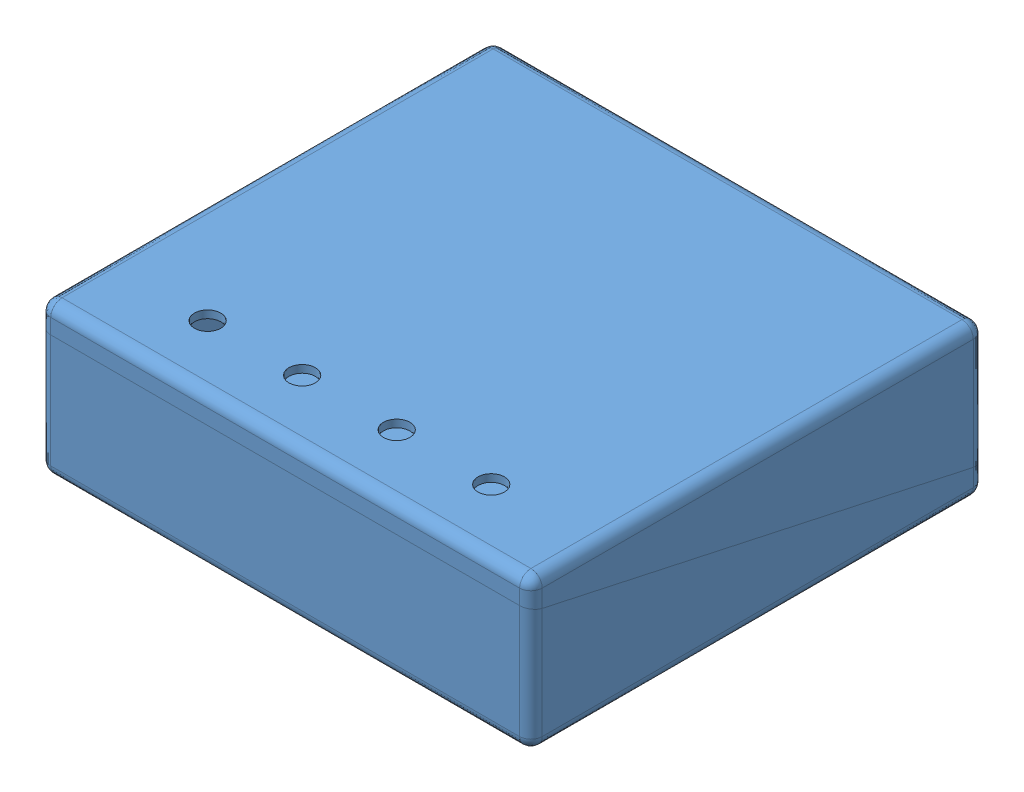
SolidWorks assembly carcasa_assembly, configuration Default. Lengths in mm.
Overall size (130 40.54 120).
283 component instances, 32 part files, 6 mates.
Components (placement in the parent):
- caracasa_amp-1: caracasa_amp [Default] at (26.1014 72.6802 108.3315) size (130 40 120)
- basic_digital1-basic_digital.step-1: basic_digital1-basic_digital.step [Default] at (-122.8986 98.8802 119.3315) x (1 0 0) z (0 1 0) size (102.24 56.26 11.54)
  - Board_Geoms_72f.step-1: Board_Geoms_72f.step [Default] at origin size (90 55 1.59)
    - Pcb_72f.step-1: Pcb_72f.step [Default] at origin size (90 55 1.59)
  - Step_Models_72f.step-1: Step_Models_72f.step [Default] at origin size (102.24 49.36 11.54)
    - Top_72f.step-1: Top_72f.step [Default] at origin size (102.24 49.36 11.54)
      - IC3_ASSEMBLY_e554ddd5023d.step-1: IC3_ASSEMBLY_e554ddd5023d.step [Default] at (179.75 26.5 0) x (0 1 0) z (0 0 1) size (5 4.4 1.3)
        - Body.step-1: Body.step [Default] at (0 0 0.1) size (5 4.4 1.2)
        - Pins.step-1: Pins.step [Default] at origin size (4.21 4.36 0.1)
      - IC1_DPD0012A_ASM_3e18ce07ad7c.step-1: IC1_DPD0012A_ASM_3e18ce07ad7c.step [Default] at (149 25.01 0.05) x (1 0 0) z (0 -1 0) size (3 0.8 3)
        - BODY-SON.step-1: BODY-SON.step [Default] at origin size (3 0.75 3)
        - FRAME-DPD0012A.step-1: FRAME-DPD0012A.step [Default] at (0 -0.05 0) size (3 0.2 3)
      - IC2_D0008A_ASM_81426aa18051.step-1: IC2_D0008A_ASM_81426aa18051.step [Default] at (131 58 0) x (0 1 0) z (0 0 1) size (6.02 4.91 1.63)
        - BODY-SO.step-1: BODY-SO.step [Default] at (0 0 1.0033) x (0 1 0) z (1 0 0) size (4.91 1.45 3.92)
        - LEAD-D0008A.step-1: LEAD-D0008A.step [Default] at (2.159 1.905 0.254) x (0 1 0) z (1 0 0) size (0.42 1 1.06)
        - LEAD-D0008A.step-2: LEAD-D0008A.step [Default] at (2.159 0.635 0.254) x (0 1 0) z (1 0 0) size (0.42 1 1.06)
        - LEAD-D0008A.step-3: LEAD-D0008A.step [Default] at (2.159 -0.635 0.254) x (0 1 0) z (1 0 0) size (0.42 1 1.06)
        - LEAD-D0008A.step-4: LEAD-D0008A.step [Default] at (2.159 -1.905 0.254) x (0 1 0) z (1 0 0) size (0.42 1 1.06)
        - LEAD-D0008A.step-5: LEAD-D0008A.step [Default] at (-2.159 1.905 0.254) x (0 -1 0) z (-1 0 0) size (0.42 1 1.06)
        - LEAD-D0008A.step-6: LEAD-D0008A.step [Default] at (-2.159 0.635 0.254) x (0 -1 0) z (-1 0 0) size (0.42 1 1.06)
        - LEAD-D0008A.step-7: LEAD-D0008A.step [Default] at (-2.159 -0.635 0.254) x (0 -1 0) z (-1 0 0) size (0.42 1 1.06)
        - LEAD-D0008A.step-8: LEAD-D0008A.step [Default] at (-2.159 -1.905 0.254) x (0 -1 0) z (-1 0 0) size (0.42 1 1.06)
      - R23_R_0603_1608Metric_a283bdbe5e44.step-1: R23_R_0603_1608Metric_a283bdbe5e44.step [Default] at (131 31.48 0) x (-1 0 0) z (0 0 1) size (1.6 0.8 0.45)
      - C52_C_0603_1608Metric_5a1a808c49e1.step-1: C52_C_0603_1608Metric_5a1a808c49e1.step [Default] at (186.25 28.5 0) x (-1 0 0) z (0 0 1) size (1.6 0.8 0.8)
      - U4_TSSOP_20_44x65mm_P065mm_811bc58fadb8.step-1: U4_TSSOP_20_44x65mm_P065mm_811bc58fadb8.step [Default] at (121.3625 24.725 0) size (6.4 6.5 1.2)
      - C52_C_0603_1608Metric_5a1a808c49e1.step-2: C52_C_0603_1608Metric_5a1a808c49e1.step [Default] at (136.75 61.25 0) x (0 1 0) z (0 0 1) size (1.6 0.8 0.8)
      - C52_C_0603_1608Metric_5a1a808c49e1.step-3: C52_C_0603_1608Metric_5a1a808c49e1.step [Default] at (151.45 44.75 0) size (1.6 0.8 0.8)
      - U7_ESP32-WROOM-32_9a0432253470.step-1: U7_ESP32-WROOM-32_9a0432253470.step [Default] at (113.495 39.92 0) x (0 1 0) z (0 0 1) size (18 25.5 3.1)
      - C52_C_0603_1608Metric_5a1a808c49e1.step-4: C52_C_0603_1608Metric_5a1a808c49e1.step [Default] at (134.25 38 0) x (0 1 0) z (0 0 1) size (1.6 0.8 0.8)
      - R23_R_0603_1608Metric_a283bdbe5e44.step-2: R23_R_0603_1608Metric_a283bdbe5e44.step [Default] at (169 35 0) size (1.6 0.8 0.45)
      - FB1_C_0805_2012Metric_4ba0fd9e626e.step-1: FB1_C_0805_2012Metric_4ba0fd9e626e.step [Default] at (150.3 56.55 0) x (-1 0 0) z (0 0 1) size (2 1.25 1.25)
      - C52_C_0603_1608Metric_5a1a808c49e1.step-5: C52_C_0603_1608Metric_5a1a808c49e1.step [Default] at (139 25.2 0) x (0 -1 0) z (0 0 1) size (1.6 0.8 0.8)
      - R23_R_0603_1608Metric_a283bdbe5e44.step-3: R23_R_0603_1608Metric_a283bdbe5e44.step [Default] at (169 36.5 0) x (-1 0 0) z (0 0 1) size (1.6 0.8 0.45)
      - R23_R_0603_1608Metric_a283bdbe5e44.step-4: R23_R_0603_1608Metric_a283bdbe5e44.step [Default] at (120.5 29 0) x (-1 0 0) z (0 0 1) size (1.6 0.8 0.45)
      - Q2_SOT_23_d2a7eeff1b69.step-1: Q2_SOT_23_d2a7eeff1b69.step [Default] at (144.75 22 0) size (2.5 3 1.2)
      - C52_C_0603_1608Metric_5a1a808c49e1.step-6: C52_C_0603_1608Metric_5a1a808c49e1.step [Default] at (159 25.25 0) x (0 1 0) z (0 0 1) size (1.6 0.8 0.8)
      - R23_R_0603_1608Metric_a283bdbe5e44.step-5: R23_R_0603_1608Metric_a283bdbe5e44.step [Default] at (132.25 46.5 0) x (-1 0 0) z (0 0 1) size (1.6 0.8 0.45)
      - FB1_C_0805_2012Metric_4ba0fd9e626e.step-2: FB1_C_0805_2012Metric_4ba0fd9e626e.step [Default] at (125.5 39 0) x (0 1 0) z (0 0 1) size (2 1.25 1.25)
      - C52_C_0603_1608Metric_5a1a808c49e1.step-7: C52_C_0603_1608Metric_5a1a808c49e1.step [Default] at (126.8625 24.975 0) x (-1 0 0) z (0 0 1) size (1.6 0.8 0.8)
      - Y1_Crystal_SMD_3225-4Pin_3.2x2.5mm_101ec78cddaa.step-1: Y1_Crystal_SMD_3225-4Pin_3.2x2.5mm_101ec78cddaa.step [Default] at (153.9 59.65 0) size (3.2 2.5 0.64)
      - J5_PinHeader_2x03_P254mm_Vertical_340915476f9a.step-1: J5_PinHeader_2x03_P254mm_Vertical_340915476f9a.step [Default] at (190.29 54.54 0) x (0 -1 0) z (0 0 1) size (5.08 7.62 11.54)
      - C52_C_0603_1608Metric_5a1a808c49e1.step-8: C52_C_0603_1608Metric_5a1a808c49e1.step [Default] at (127.98 32.98 0) x (-1 0 0) z (0 0 1) size (1.6 0.8 0.8)
      - C52_C_0603_1608Metric_5a1a808c49e1.step-9: C52_C_0603_1608Metric_5a1a808c49e1.step [Default] at (149.75 28.45 0) x (0 1 0) z (0 0 1) size (1.6 0.8 0.8)
      - C52_C_0603_1608Metric_5a1a808c49e1.step-10: C52_C_0603_1608Metric_5a1a808c49e1.step [Default] at (126.8625 26.475 0) x (-1 0 0) z (0 0 1) size (1.6 0.8 0.8)
      - C52_C_0603_1608Metric_5a1a808c49e1.step-11: C52_C_0603_1608Metric_5a1a808c49e1.step [Default] at (138.25 58.25 0) x (0 -1 0) z (0 0 1) size (1.6 0.8 0.8)
      - C52_C_0603_1608Metric_5a1a808c49e1.step-12: C52_C_0603_1608Metric_5a1a808c49e1.step [Default] at (162.3 49.05 0) x (-1 0 0) z (0 0 1) size (1.6 0.8 0.8)
      - R23_R_0603_1608Metric_a283bdbe5e44.step-6: R23_R_0603_1608Metric_a283bdbe5e44.step [Default] at (193 54.75 0) x (0 -1 0) z (0 0 1) size (1.6 0.8 0.45)
      - R23_R_0603_1608Metric_a283bdbe5e44.step-7: R23_R_0603_1608Metric_a283bdbe5e44.step [Default] at (167.5 47.25 0) x (-1 0 0) z (0 0 1) size (1.6 0.8 0.45)
      - D1_D_SOD_123_ffc0e81b88b9.step-1: D1_D_SOD_123_ffc0e81b88b9.step [Default] at (127 64.25 0) x (0 1 0) z (0 0 1) size (3.8 1.6 1.25)
      - R23_R_0603_1608Metric_a283bdbe5e44.step-8: R23_R_0603_1608Metric_a283bdbe5e44.step [Default] at (170.5 47.25 0) size (1.6 0.8 0.45)
      - C52_C_0603_1608Metric_5a1a808c49e1.step-13: C52_C_0603_1608Metric_5a1a808c49e1.step [Default] at (139 21.95 0) x (0 -1 0) z (0 0 1) size (1.6 0.8 0.8)
      - R23_R_0603_1608Metric_a283bdbe5e44.step-9: R23_R_0603_1608Metric_a283bdbe5e44.step [Default] at (169.75 32.75 0) x (0 1 0) z (0 0 1) size (1.6 0.8 0.45)
      - Q2_SOT_23_d2a7eeff1b69.step-2: Q2_SOT_23_d2a7eeff1b69.step [Default] at (153.25 22 0) x (-1 0 0) z (0 0 1) size (2.5 3 1.2)
      - R23_R_0603_1608Metric_a283bdbe5e44.step-10: R23_R_0603_1608Metric_a283bdbe5e44.step [Default] at (190 28.5 0) x (0 1 0) z (0 0 1) size (1.6 0.8 0.45)
      - C52_C_0603_1608Metric_5a1a808c49e1.step-14: C52_C_0603_1608Metric_5a1a808c49e1.step [Default] at (155.45 42.4 0) x (0 -1 0) z (0 0 1) size (1.6 0.8 0.8)
      - C52_C_0603_1608Metric_5a1a808c49e1.step-15: C52_C_0603_1608Metric_5a1a808c49e1.step [Default] at (114.3375 28.475 0) size (1.6 0.8 0.8)
      - R23_R_0603_1608Metric_a283bdbe5e44.step-11: R23_R_0603_1608Metric_a283bdbe5e44.step [Default] at (131.5 44.25 0) x (0 1 0) z (0 0 1) size (1.6 0.8 0.45)
      - R23_R_0603_1608Metric_a283bdbe5e44.step-12: R23_R_0603_1608Metric_a283bdbe5e44.step [Default] at (182.5 51.5 0) x (0 -1 0) z (0 0 1) size (1.6 0.8 0.45)
      - C52_C_0603_1608Metric_5a1a808c49e1.step-16: C52_C_0603_1608Metric_5a1a808c49e1.step [Default] at (171.25 32.75 0) x (0 -1 0) z (0 0 1) size (1.6 0.8 0.8)
      - C52_C_0603_1608Metric_5a1a808c49e1.step-17: C52_C_0603_1608Metric_5a1a808c49e1.step [Default] at (141.5 55.75 0) x (0 1 0) z (0 0 1) size (1.6 0.8 0.8)
      - R23_R_0603_1608Metric_a283bdbe5e44.step-13: R23_R_0603_1608Metric_a283bdbe5e44.step [Default] at (170 58.5 0) size (1.6 0.8 0.45)
      - C52_C_0603_1608Metric_5a1a808c49e1.step-18: C52_C_0603_1608Metric_5a1a808c49e1.step [Default] at (168.25 32.75 0) x (0 1 0) z (0 0 1) size (1.6 0.8 0.8)
      - R23_R_0603_1608Metric_a283bdbe5e44.step-14: R23_R_0603_1608Metric_a283bdbe5e44.step [Default] at (160.75 64.75 0) size (1.6 0.8 0.45)
      - C52_C_0603_1608Metric_5a1a808c49e1.step-19: C52_C_0603_1608Metric_5a1a808c49e1.step [Default] at (154.35 56.05 0) x (0 -1 0) z (0 0 1) size (1.6 0.8 0.8)
      - R23_R_0603_1608Metric_a283bdbe5e44.step-15: R23_R_0603_1608Metric_a283bdbe5e44.step [Default] at (170.5 48.75 0) x (-1 0 0) z (0 0 1) size (1.6 0.8 0.45)
      - R23_R_0603_1608Metric_a283bdbe5e44.step-16: R23_R_0603_1608Metric_a283bdbe5e44.step [Default] at (167.5 45.75 0) size (1.6 0.8 0.45)
      - C52_C_0603_1608Metric_5a1a808c49e1.step-20: C52_C_0603_1608Metric_5a1a808c49e1.step [Default] at (119 55.75 0) x (0 -1 0) z (0 0 1) size (1.6 0.8 0.8)
      - R23_R_0603_1608Metric_a283bdbe5e44.step-17: R23_R_0603_1608Metric_a283bdbe5e44.step [Default] at (130.25 33.75 0) x (0 -1 0) z (0 0 1) size (1.6 0.8 0.45)
      - C52_C_0603_1608Metric_5a1a808c49e1.step-21: C52_C_0603_1608Metric_5a1a808c49e1.step [Default] at (153.95 42.4 0) x (0 -1 0) z (0 0 1) size (1.6 0.8 0.8)
      - C52_C_0603_1608Metric_5a1a808c49e1.step-22: C52_C_0603_1608Metric_5a1a808c49e1.step [Default] at (142 25.2 0) x (0 1 0) z (0 0 1) size (1.6 0.8 0.8)
      - C52_C_0603_1608Metric_5a1a808c49e1.step-23: C52_C_0603_1608Metric_5a1a808c49e1.step [Default] at (126.8625 27.975 0) x (-1 0 0) z (0 0 1) size (1.6 0.8 0.8)
      - R23_R_0603_1608Metric_a283bdbe5e44.step-18: R23_R_0603_1608Metric_a283bdbe5e44.step [Default] at (170 64.5 0) size (1.6 0.8 0.45)
      - C52_C_0603_1608Metric_5a1a808c49e1.step-24: C52_C_0603_1608Metric_5a1a808c49e1.step [Default] at (150.51 21.5 0) x (0 1 0) z (0 0 1) size (1.6 0.8 0.8)
      - J2_PinHeader_1x05_P254mm_Vertical_afd68b060886.step-1: J2_PinHeader_1x05_P254mm_Vertical_afd68b060886.step [Default] at (154.04 64.5 0) x (0 -1 0) z (0 0 1) size (2.54 12.7 11.54)
      - C52_C_0603_1608Metric_5a1a808c49e1.step-25: C52_C_0603_1608Metric_5a1a808c49e1.step [Default] at (161.45 42.4 0) x (0 1 0) z (0 0 1) size (1.6 0.8 0.8)
      - C52_C_0603_1608Metric_5a1a808c49e1.step-26: C52_C_0603_1608Metric_5a1a808c49e1.step [Default] at (105.75 28.75 0) x (-1 0 0) z (0 0 1) size (1.6 0.8 0.8)
      - U1_LQFP_48_7x7mm_P05mm_03b825850876.step-1: U1_LQFP_48_7x7mm_P05mm_03b825850876.step [Default] at (163 58.5 0) size (9 9 1.5)
      - R23_R_0603_1608Metric_a283bdbe5e44.step-19: R23_R_0603_1608Metric_a283bdbe5e44.step [Default] at (134.6 64.825 0) x (0 1 0) z (0 0 1) size (1.6 0.8 0.45)
      - C52_C_0603_1608Metric_5a1a808c49e1.step-27: C52_C_0603_1608Metric_5a1a808c49e1.step [Default] at (172.75 49.5 0) x (0 -1 0) z (0 0 1) size (1.6 0.8 0.8)
      - C52_C_0603_1608Metric_5a1a808c49e1.step-28: C52_C_0603_1608Metric_5a1a808c49e1.step [Default] at (168 53.75 0) size (1.6 0.8 0.8)
      - R23_R_0603_1608Metric_a283bdbe5e44.step-20: R23_R_0603_1608Metric_a283bdbe5e44.step [Default] at (125.25 20.2 0) size (1.6 0.8 0.45)
      - C52_C_0603_1608Metric_5a1a808c49e1.step-29: C52_C_0603_1608Metric_5a1a808c49e1.step [Default] at (193 51.5 0) x (0 -1 0) z (0 0 1) size (1.6 0.8 0.8)
      - R23_R_0603_1608Metric_a283bdbe5e44.step-21: R23_R_0603_1608Metric_a283bdbe5e44.step [Default] at (170.5 50.25 0) x (-1 0 0) z (0 0 1) size (1.6 0.8 0.45)
      - C52_C_0603_1608Metric_5a1a808c49e1.step-30: C52_C_0603_1608Metric_5a1a808c49e1.step [Default] at (168.25 49.5 0) x (0 1 0) z (0 0 1) size (1.6 0.8 0.8)
      - C52_C_0603_1608Metric_5a1a808c49e1.step-31: C52_C_0603_1608Metric_5a1a808c49e1.step [Default] at (116.5875 27.725 0) x (0 1 0) z (0 0 1) size (1.6 0.8 0.8)
      - R23_R_0603_1608Metric_a283bdbe5e44.step-22: R23_R_0603_1608Metric_a283bdbe5e44.step [Default] at (159.95 42.4 0) x (0 -1 0) z (0 0 1) size (1.6 0.8 0.45)
      - R23_R_0603_1608Metric_a283bdbe5e44.step-23: R23_R_0603_1608Metric_a283bdbe5e44.step [Default] at (105 52.25 0) x (0 -1 0) z (0 0 1) size (1.6 0.8 0.45)
      - C52_C_0603_1608Metric_5a1a808c49e1.step-32: C52_C_0603_1608Metric_5a1a808c49e1.step [Default] at (151.45 49.4 0) x (-1 0 0) z (0 0 1) size (1.6 0.8 0.8)
      - R23_R_0603_1608Metric_a283bdbe5e44.step-24: R23_R_0603_1608Metric_a283bdbe5e44.step [Default] at (157.5 22.25 0) x (0 -1 0) z (0 0 1) size (1.6 0.8 0.45)
      - R23_R_0603_1608Metric_a283bdbe5e44.step-25: R23_R_0603_1608Metric_a283bdbe5e44.step [Default] at (108.25 28 0) x (0 -1 0) z (0 0 1) size (1.6 0.8 0.45)
      - C52_C_0603_1608Metric_5a1a808c49e1.step-33: C52_C_0603_1608Metric_5a1a808c49e1.step [Default] at (155.85 56.05 0) x (0 -1 0) z (0 0 1) size (1.6 0.8 0.8)
      - C52_C_0603_1608Metric_5a1a808c49e1.step-34: C52_C_0603_1608Metric_5a1a808c49e1.step [Default] at (181.75 20.75 0) size (1.6 0.8 0.8)
      - C52_C_0603_1608Metric_5a1a808c49e1.step-35: C52_C_0603_1608Metric_5a1a808c49e1.step [Default] at (159.2 39.9 0) x (-1 0 0) z (0 0 1) size (1.6 0.8 0.8)
      - R23_R_0603_1608Metric_a283bdbe5e44.step-26: R23_R_0603_1608Metric_a283bdbe5e44.step [Default] at (170.5 45.75 0) x (-1 0 0) z (0 0 1) size (1.6 0.8 0.45)
      - R23_R_0603_1608Metric_a283bdbe5e44.step-27: R23_R_0603_1608Metric_a283bdbe5e44.step [Default] at (144.25 24.5 0) x (-1 0 0) z (0 0 1) size (1.6 0.8 0.45)
      - C15_C_1206_3216Metric_52626895d937.step-1: C15_C_1206_3216Metric_52626895d937.step [Default] at (121 55 0) x (0 -1 0) z (0 0 1) size (3.2 1.6 1.6)
      - C52_C_0603_1608Metric_5a1a808c49e1.step-36: C52_C_0603_1608Metric_5a1a808c49e1.step [Default] at (173.75 24.25 0) x (-1 0 0) z (0 0 1) size (1.6 0.8 0.8)
      - C52_C_0603_1608Metric_5a1a808c49e1.step-37: C52_C_0603_1608Metric_5a1a808c49e1.step [Default] at (150.4 42.15 0) x (0 1 0) z (0 0 1) size (1.6 0.8 0.8)
      - R23_R_0603_1608Metric_a283bdbe5e44.step-28: R23_R_0603_1608Metric_a283bdbe5e44.step [Default] at (170 66 0) size (1.6 0.8 0.45)
      - C52_C_0603_1608Metric_5a1a808c49e1.step-38: C52_C_0603_1608Metric_5a1a808c49e1.step [Default] at (115.8375 22.475 0) size (1.6 0.8 0.8)
      - R23_R_0603_1608Metric_a283bdbe5e44.step-29: R23_R_0603_1608Metric_a283bdbe5e44.step [Default] at (133.1 64.9 0) x (0 1 0) z (0 0 1) size (1.6 0.8 0.45)
      - U5_SOIC_8_39x49mm_P127mm_56764403cdee.step-1: U5_SOIC_8_39x49mm_P127mm_56764403cdee.step [Default] at (129.25 39 0) x (0 1 0) z (0 0 1) size (6 4.9 1.75)
      - C52_C_0603_1608Metric_5a1a808c49e1.step-39: C52_C_0603_1608Metric_5a1a808c49e1.step [Default] at (127 60 0) x (0 -1 0) z (0 0 1) size (1.6 0.8 0.8)
      - C52_C_0603_1608Metric_5a1a808c49e1.step-40: C52_C_0603_1608Metric_5a1a808c49e1.step [Default] at (146.25 61 0) x (0 -1 0) z (0 0 1) size (1.6 0.8 0.8)
      - C52_C_0603_1608Metric_5a1a808c49e1.step-41: C52_C_0603_1608Metric_5a1a808c49e1.step [Default] at (115.8375 23.975 0) size (1.6 0.8 0.8)
      - C52_C_0603_1608Metric_5a1a808c49e1.step-42: C52_C_0603_1608Metric_5a1a808c49e1.step [Default] at (157.5 25.25 0) x (0 1 0) z (0 0 1) size (1.6 0.8 0.8)
      - R23_R_0603_1608Metric_a283bdbe5e44.step-30: R23_R_0603_1608Metric_a283bdbe5e44.step [Default] at (170 61.5 0) size (1.6 0.8 0.45)
      - C52_C_0603_1608Metric_5a1a808c49e1.step-43: C52_C_0603_1608Metric_5a1a808c49e1.step [Default] at (173.75 25.75 0) x (-1 0 0) z (0 0 1) size (1.6 0.8 0.8)
      - J1_12401610E42A_e582b0f26147.step-1: J1_12401610E42A_e582b0f26147.step [Default] at (177.5 68.25 1.55) x (0 1 0) z (0 0 1) size (10.51 9.21 4.22)
      - C52_C_0603_1608Metric_5a1a808c49e1.step-44: C52_C_0603_1608Metric_5a1a808c49e1.step [Default] at (186.25 27 0) x (-1 0 0) z (0 0 1) size (1.6 0.8 0.8)
      - C52_C_0603_1608Metric_5a1a808c49e1.step-45: C52_C_0603_1608Metric_5a1a808c49e1.step [Default] at (156 25.25 0) x (0 1 0) z (0 0 1) size (1.6 0.8 0.8)
      - R23_R_0603_1608Metric_a283bdbe5e44.step-31: R23_R_0603_1608Metric_a283bdbe5e44.step [Default] at (129.25 46.48 0) size (1.6 0.8 0.45)
      - C52_C_0603_1608Metric_5a1a808c49e1.step-46: C52_C_0603_1608Metric_5a1a808c49e1.step [Default] at (158.5 64 0) x (0 1 0) z (0 0 1) size (1.6 0.8 0.8)
      - C52_C_0603_1608Metric_5a1a808c49e1.step-47: C52_C_0603_1608Metric_5a1a808c49e1.step [Default] at (156 22.25 0) x (0 -1 0) z (0 0 1) size (1.6 0.8 0.8)
      - R23_R_0603_1608Metric_a283bdbe5e44.step-32: R23_R_0603_1608Metric_a283bdbe5e44.step [Default] at (157 64 0) x (0 -1 0) z (0 0 1) size (1.6 0.8 0.45)
      - C52_C_0603_1608Metric_5a1a808c49e1.step-48: C52_C_0603_1608Metric_5a1a808c49e1.step [Default] at (136.75 58.25 0) x (0 -1 0) z (0 0 1) size (1.6 0.8 0.8)
      - R23_R_0603_1608Metric_a283bdbe5e44.step-33: R23_R_0603_1608Metric_a283bdbe5e44.step [Default] at (156.85 59.5 0) x (0 -1 0) z (0 0 1) size (1.6 0.8 0.45)
      - R23_R_0603_1608Metric_a283bdbe5e44.step-34: R23_R_0603_1608Metric_a283bdbe5e44.step [Default] at (134.6 61.825 0) x (0 1 0) z (0 0 1) size (1.6 0.8 0.45)
      - C52_C_0603_1608Metric_5a1a808c49e1.step-49: C52_C_0603_1608Metric_5a1a808c49e1.step [Default] at (134.6 55.65 0) x (0 1 0) z (0 0 1) size (1.6 0.8 0.8)
      - C52_C_0603_1608Metric_5a1a808c49e1.step-50: C52_C_0603_1608Metric_5a1a808c49e1.step [Default] at (132.35 62.65 0) size (1.6 0.8 0.8)
      - R23_R_0603_1608Metric_a283bdbe5e44.step-35: R23_R_0603_1608Metric_a283bdbe5e44.step [Default] at (171.25 35.75 0) x (0 -1 0) z (0 0 1) size (1.6 0.8 0.45)
      - C52_C_0603_1608Metric_5a1a808c49e1.step-51: C52_C_0603_1608Metric_5a1a808c49e1.step [Default] at (133 44.25 0) x (0 1 0) z (0 0 1) size (1.6 0.8 0.8)
      - J5_PinHeader_2x03_P254mm_Vertical_340915476f9a.step-2: J5_PinHeader_2x03_P254mm_Vertical_340915476f9a.step [Default] at (107.725 52.475 0) x (0 1 0) z (0 0 1) size (5.08 7.62 11.54)
      - R23_R_0603_1608Metric_a283bdbe5e44.step-36: R23_R_0603_1608Metric_a283bdbe5e44.step [Default] at (158.45 42.4 0) x (0 1 0) z (0 0 1) size (1.6 0.8 0.45)
      - U7_ESP32-WROOM-32_9a0432253470.step-2: U7_ESP32-WROOM-32_9a0432253470.step [Default] at (184.245 40 0) x (0 -1 0) z (0 0 1) size (18 25.5 3.1)
      - U3_UQFN-16-1EP_3x3mm_Pitch0.5mm_2c02add8b7c8.step-1: U3_UQFN-16-1EP_3x3mm_Pitch0.5mm_2c02add8b7c8.step [Default] at (142 60 0) x (-1 0 0) z (0 0 1) size (3 3 0.52)
      - C52_C_0603_1608Metric_5a1a808c49e1.step-52: C52_C_0603_1608Metric_5a1a808c49e1.step [Default] at (147.5 21.5 0) x (0 1 0) z (0 0 1) size (1.6 0.8 0.8)
      - C52_C_0603_1608Metric_5a1a808c49e1.step-53: C52_C_0603_1608Metric_5a1a808c49e1.step [Default] at (131.75 33.75 0) x (0 -1 0) z (0 0 1) size (1.6 0.8 0.8)
      - C52_C_0603_1608Metric_5a1a808c49e1.step-54: C52_C_0603_1608Metric_5a1a808c49e1.step [Default] at (138.25 61.25 0) x (0 1 0) z (0 0 1) size (1.6 0.8 0.8)
      - R23_R_0603_1608Metric_a283bdbe5e44.step-37: R23_R_0603_1608Metric_a283bdbe5e44.step [Default] at (128 31.5 0) size (1.6 0.8 0.45)
      - R23_R_0603_1608Metric_a283bdbe5e44.step-38: R23_R_0603_1608Metric_a283bdbe5e44.step [Default] at (151.45 46.4 0) x (-1 0 0) z (0 0 1) size (1.6 0.8 0.45)
      - U5_SOIC_8_39x49mm_P127mm_56764403cdee.step-2: U5_SOIC_8_39x49mm_P127mm_56764403cdee.step [Default] at (157 47 0) size (6 4.9 1.75)
      - C52_C_0603_1608Metric_5a1a808c49e1.step-55: C52_C_0603_1608Metric_5a1a808c49e1.step [Default] at (131.6 64.9 0) x (0 1 0) z (0 0 1) size (1.6 0.8 0.8)
      - C52_C_0603_1608Metric_5a1a808c49e1.step-56: C52_C_0603_1608Metric_5a1a808c49e1.step [Default] at (126.8625 23.475 0) x (-1 0 0) z (0 0 1) size (1.6 0.8 0.8)
      - C52_C_0603_1608Metric_5a1a808c49e1.step-57: C52_C_0603_1608Metric_5a1a808c49e1.step [Default] at (186.25 23.75 0) x (-1 0 0) z (0 0 1) size (1.6 0.8 0.8)
      - R23_R_0603_1608Metric_a283bdbe5e44.step-39: R23_R_0603_1608Metric_a283bdbe5e44.step [Default] at (126.8625 21.75 0) size (1.6 0.8 0.45)
      - C52_C_0603_1608Metric_5a1a808c49e1.step-58: C52_C_0603_1608Metric_5a1a808c49e1.step [Default] at (150.2 58.8 0) size (1.6 0.8 0.8)
      - C52_C_0603_1608Metric_5a1a808c49e1.step-59: C52_C_0603_1608Metric_5a1a808c49e1.step [Default] at (164.75 42 0) x (-1 0 0) z (0 0 1) size (1.6 0.8 0.8)
      - R23_R_0603_1608Metric_a283bdbe5e44.step-40: R23_R_0603_1608Metric_a283bdbe5e44.step [Default] at (140.5 25.2 0) x (0 1 0) z (0 0 1) size (1.6 0.8 0.45)
      - FB1_C_0805_2012Metric_4ba0fd9e626e.step-3: FB1_C_0805_2012Metric_4ba0fd9e626e.step [Default] at (152.2 42.15 0) x (0 -1 0) z (0 0 1) size (2 1.25 1.25)
      - C52_C_0603_1608Metric_5a1a808c49e1.step-60: C52_C_0603_1608Metric_5a1a808c49e1.step [Default] at (132.75 38 0) x (0 1 0) z (0 0 1) size (1.6 0.8 0.8)
      - R23_R_0603_1608Metric_a283bdbe5e44.step-41: R23_R_0603_1608Metric_a283bdbe5e44.step [Default] at (143 55.75 0) x (0 1 0) z (0 0 1) size (1.6 0.8 0.45)
      - C52_C_0603_1608Metric_5a1a808c49e1.step-61: C52_C_0603_1608Metric_5a1a808c49e1.step [Default] at (129.25 44.98 0) x (-1 0 0) z (0 0 1) size (1.6 0.8 0.8)
      - R23_R_0603_1608Metric_a283bdbe5e44.step-42: R23_R_0603_1608Metric_a283bdbe5e44.step [Default] at (144.5 55.75 0) x (0 -1 0) z (0 0 1) size (1.6 0.8 0.45)
      - C52_C_0603_1608Metric_5a1a808c49e1.step-62: C52_C_0603_1608Metric_5a1a808c49e1.step [Default] at (164.75 40.5 0) x (-1 0 0) z (0 0 1) size (1.6 0.8 0.8)
      - C52_C_0603_1608Metric_5a1a808c49e1.step-63: C52_C_0603_1608Metric_5a1a808c49e1.step [Default] at (181.75 22.25 0) size (1.6 0.8 0.8)
      - C15_C_1206_3216Metric_52626895d937.step-2: C15_C_1206_3216Metric_52626895d937.step [Default] at (123.5 55 0) x (0 -1 0) z (0 0 1) size (3.2 1.6 1.6)
      - C52_C_0603_1608Metric_5a1a808c49e1.step-64: C52_C_0603_1608Metric_5a1a808c49e1.step [Default] at (159 22.25 0) x (0 -1 0) z (0 0 1) size (1.6 0.8 0.8)
      - R23_R_0603_1608Metric_a283bdbe5e44.step-43: R23_R_0603_1608Metric_a283bdbe5e44.step [Default] at (170 60 0) size (1.6 0.8 0.45)
      - C52_C_0603_1608Metric_5a1a808c49e1.step-65: C52_C_0603_1608Metric_5a1a808c49e1.step [Default] at (114.3375 26.975 0) size (1.6 0.8 0.8)
      - C52_C_0603_1608Metric_5a1a808c49e1.step-66: C52_C_0603_1608Metric_5a1a808c49e1.step [Default] at (170 63 0) size (1.6 0.8 0.8)
      - R23_R_0603_1608Metric_a283bdbe5e44.step-44: R23_R_0603_1608Metric_a283bdbe5e44.step [Default] at (166 36.5 0) size (1.6 0.8 0.45)
      - C52_C_0603_1608Metric_5a1a808c49e1.step-67: C52_C_0603_1608Metric_5a1a808c49e1.step [Default] at (172.5 40.25 0) x (0 1 0) z (0 0 1) size (1.6 0.8 0.8)
      - C52_C_0603_1608Metric_5a1a808c49e1.step-68: C52_C_0603_1608Metric_5a1a808c49e1.step [Default] at (142 21.95 0) x (0 -1 0) z (0 0 1) size (1.6 0.8 0.8)
      - U5_SOIC_8_39x49mm_P127mm_56764403cdee.step-3: U5_SOIC_8_39x49mm_P127mm_56764403cdee.step [Default] at (169 41.25 0) x (0 -1 0) z (0 0 1) size (6 4.9 1.75)
      - C52_C_0603_1608Metric_5a1a808c49e1.step-69: C52_C_0603_1608Metric_5a1a808c49e1.step [Default] at (153.75 26 0) size (1.6 0.8 0.8)
      - R23_R_0603_1608Metric_a283bdbe5e44.step-45: R23_R_0603_1608Metric_a283bdbe5e44.step [Default] at (151.45 47.9 0) size (1.6 0.8 0.45)
      - C52_C_0603_1608Metric_5a1a808c49e1.step-70: C52_C_0603_1608Metric_5a1a808c49e1.step [Default] at (152.85 56.05 0) x (0 -1 0) z (0 0 1) size (1.6 0.8 0.8)
      - R23_R_0603_1608Metric_a283bdbe5e44.step-46: R23_R_0603_1608Metric_a283bdbe5e44.step [Default] at (166 35 0) x (-1 0 0) z (0 0 1) size (1.6 0.8 0.45)
      - R23_R_0603_1608Metric_a283bdbe5e44.step-47: R23_R_0603_1608Metric_a283bdbe5e44.step [Default] at (156.375 50.65 0) x (-1 0 0) z (0 0 1) size (1.6 0.8 0.45)
      - C52_C_0603_1608Metric_5a1a808c49e1.step-71: C52_C_0603_1608Metric_5a1a808c49e1.step [Default] at (149.01 21.5 0) x (0 1 0) z (0 0 1) size (1.6 0.8 0.8)
      - R23_R_0603_1608Metric_a283bdbe5e44.step-48: R23_R_0603_1608Metric_a283bdbe5e44.step [Default] at (153.75 24.5 0) size (1.6 0.8 0.45)
      - C52_C_0603_1608Metric_5a1a808c49e1.step-72: C52_C_0603_1608Metric_5a1a808c49e1.step [Default] at (140.5 21.95 0) x (0 -1 0) z (0 0 1) size (1.6 0.8 0.8)
      - C52_C_0603_1608Metric_5a1a808c49e1.step-73: C52_C_0603_1608Metric_5a1a808c49e1.step [Default] at (115.8375 25.475 0) size (1.6 0.8 0.8)
      - R23_R_0603_1608Metric_a283bdbe5e44.step-49: R23_R_0603_1608Metric_a283bdbe5e44.step [Default] at (140 55.75 0) x (0 -1 0) z (0 0 1) size (1.6 0.8 0.45)
      - C52_C_0603_1608Metric_5a1a808c49e1.step-74: C52_C_0603_1608Metric_5a1a808c49e1.step [Default] at (144.25 26 0) x (-1 0 0) z (0 0 1) size (1.6 0.8 0.8)
      - C52_C_0603_1608Metric_5a1a808c49e1.step-75: C52_C_0603_1608Metric_5a1a808c49e1.step [Default] at (148.25 28.45 0) x (0 1 0) z (0 0 1) size (1.6 0.8 0.8)
      - C52_C_0603_1608Metric_5a1a808c49e1.step-76: C52_C_0603_1608Metric_5a1a808c49e1.step [Default] at (150.2 60.5 0) size (1.6 0.8 0.8)
      - C52_C_0603_1608Metric_5a1a808c49e1.step-77: C52_C_0603_1608Metric_5a1a808c49e1.step [Default] at (156.95 42.4 0) x (0 -1 0) z (0 0 1) size (1.6 0.8 0.8)
      - R23_R_0603_1608Metric_a283bdbe5e44.step-50: R23_R_0603_1608Metric_a283bdbe5e44.step [Default] at (120.9 19.7 0) x (0 1 0) z (0 0 1) size (1.6 0.8 0.45)
      - C52_C_0603_1608Metric_5a1a808c49e1.step-78: C52_C_0603_1608Metric_5a1a808c49e1.step [Default] at (186.25 25.25 0) x (-1 0 0) z (0 0 1) size (1.6 0.8 0.8)
      - R23_R_0603_1608Metric_a283bdbe5e44.step-51: R23_R_0603_1608Metric_a283bdbe5e44.step [Default] at (122.4 19.7 0) x (0 1 0) z (0 0 1) size (1.6 0.8 0.45)
- analog_board-analog_board.step-1: analog_board-analog_board.step [Default] at (-128.8986 82.2702 -20.6685) x (1 0 0) z (0 1 0) size (90 58.5 20.63)
  - Board_Geoms_11b5.step-1: Board_Geoms_11b5.step [Default] at origin size (90 55 1.59)
    - Pcb_11b5.step-1: Pcb_11b5.step [Default] at origin size (90 55 1.59)
  - Step_Models_11b5.step-1: Step_Models_11b5.step [Default] at origin size (67.77 53.9 20.63)
    - Top_11b5.step-1: Top_11b5.step [Default] at origin size (67.65 53.9 11.3)
      - R37_R_0603_1608Metric_000060c15df4.step-1: R37_R_0603_1608Metric_000060c15df4.step [Default] at (132.15 -103.5255 0) x (0 -1 0) z (0 0 1) size (1.6 0.8 0.45)
      - R37_R_0603_1608Metric_000060c15df4.step-2: R37_R_0603_1608Metric_000060c15df4.step [Default] at (129.15 -103.5255 0) x (0 -1 0) z (0 0 1) size (1.6 0.8 0.45)
      - R37_R_0603_1608Metric_000060c15df4.step-3: R37_R_0603_1608Metric_000060c15df4.step [Default] at (124.65 -103.5255 0) x (0 -1 0) z (0 0 1) size (1.6 0.8 0.45)
      - R37_R_0603_1608Metric_000060c15df4.step-4: R37_R_0603_1608Metric_000060c15df4.step [Default] at (123.15 -103.5255 0) x (0 -1 0) z (0 0 1) size (1.6 0.8 0.45)
      - R37_R_0603_1608Metric_000060c15df4.step-5: R37_R_0603_1608Metric_000060c15df4.step [Default] at (124.25 -91.5 0) size (1.6 0.8 0.45)
      - R37_R_0603_1608Metric_000060c15df4.step-6: R37_R_0603_1608Metric_000060c15df4.step [Default] at (135.6 -92.9 0) x (-1 0 0) z (0 0 1) size (1.6 0.8 0.45)
      - R37_R_0603_1608Metric_000060c15df4.step-7: R37_R_0603_1608Metric_000060c15df4.step [Default] at (121.65 -103.5255 0) x (0 -1 0) z (0 0 1) size (1.6 0.8 0.45)
      - R37_R_0603_1608Metric_000060c15df4.step-8: R37_R_0603_1608Metric_000060c15df4.step [Default] at (126.15 -103.5255 0) x (0 -1 0) z (0 0 1) size (1.6 0.8 0.45)
      - R37_R_0603_1608Metric_000060c15df4.step-9: R37_R_0603_1608Metric_000060c15df4.step [Default] at (127.65 -103.5255 0) x (0 -1 0) z (0 0 1) size (1.6 0.8 0.45)
      - R37_R_0603_1608Metric_000060c15df4.step-10: R37_R_0603_1608Metric_000060c15df4.step [Default] at (130.65 -103.5255 0) x (0 -1 0) z (0 0 1) size (1.6 0.8 0.45)
      - U3_SOIC_8_39x49mm_P127mm_000060c16360.step-1: U3_SOIC_8_39x49mm_P127mm_000060c16360.step [Default] at (130 -93.5 0) size (6 4.9 1.75)
      - C33_C_0603_1608Metric_000060c4abf8.step-1: C33_C_0603_1608Metric_000060c4abf8.step [Default] at (129.75 -97.25 0) x (-1 0 0) z (0 0 1) size (1.6 0.8 0.8)
      - Q1_SOT_23_000060c531eb.step-1: Q1_SOT_23_000060c531eb.step [Default] at (181.25 -101.25 0) x (-1 0 0) z (0 0 1) size (2.5 3 1.2)
      - Q1_SOT_23_000060c531eb.step-2: Q1_SOT_23_000060c531eb.step [Default] at (177.5 -101.25 0) size (2.5 3 1.2)
      - R37_R_0603_1608Metric_000060c15df4.step-11: R37_R_0603_1608Metric_000060c15df4.step [Default] at (174 -102.25 0) size (1.6 0.8 0.45)
      - R37_R_0603_1608Metric_000060c15df4.step-12: R37_R_0603_1608Metric_000060c15df4.step [Default] at (174 -104.25 0) x (-1 0 0) z (0 0 1) size (1.6 0.8 0.45)
      - R37_R_0603_1608Metric_000060c15df4.step-13: R37_R_0603_1608Metric_000060c15df4.step [Default] at (174 -100.25 0) x (-1 0 0) z (0 0 1) size (1.6 0.8 0.45)
      - R37_R_0603_1608Metric_000060c15df4.step-14: R37_R_0603_1608Metric_000060c15df4.step [Default] at (174 -106.25 0) x (-1 0 0) z (0 0 1) size (1.6 0.8 0.45)
      - R37_R_0603_1608Metric_000060c15df4.step-15: R37_R_0603_1608Metric_000060c15df4.step [Default] at (184.75 -101.75 0) x (-1 0 0) z (0 0 1) size (1.6 0.8 0.45)
      - R37_R_0603_1608Metric_000060c15df4.step-16: R37_R_0603_1608Metric_000060c15df4.step [Default] at (184.75 -100.25 0) size (1.6 0.8 0.45)
      - R37_R_0603_1608Metric_000060c15df4.step-17: R37_R_0603_1608Metric_000060c15df4.step [Default] at (184.75 -103.25 0) size (1.6 0.8 0.45)
      - R37_R_0603_1608Metric_000060c15df4.step-18: R37_R_0603_1608Metric_000060c15df4.step [Default] at (184.75 -104.75 0) size (1.6 0.8 0.45)
      - C7_CP_Elec_8x105_000060c673e7.step-1: C7_CP_Elec_8x105_000060c673e7.step [Default] at (177.75 -94.75 0) size (10.73 10.93 10.5)
      - R37_R_0603_1608Metric_000060c15df4.step-19: R37_R_0603_1608Metric_000060c15df4.step [Default] at (177.975 -109.5 0) x (0 -1 0) z (0 0 1) size (1.6 0.8 0.45)
      - R37_R_0603_1608Metric_000060c15df4.step-20: R37_R_0603_1608Metric_000060c15df4.step [Default] at (188.5 -93.75 0) x (0 -1 0) z (0 0 1) size (1.6 0.8 0.45)
      - R37_R_0603_1608Metric_000060c15df4.step-21: R37_R_0603_1608Metric_000060c15df4.step [Default] at (177.225 -112 0) x (-1 0 0) z (0 0 1) size (1.6 0.8 0.45)
      - R37_R_0603_1608Metric_000060c15df4.step-22: R37_R_0603_1608Metric_000060c15df4.step [Default] at (184.75 -106.25 0) size (1.6 0.8 0.45)
      - R37_R_0603_1608Metric_000060c15df4.step-23: R37_R_0603_1608Metric_000060c15df4.step [Default] at (177.225 -113.75 0) size (1.6 0.8 0.45)
      - R37_R_0603_1608Metric_000060c15df4.step-24: R37_R_0603_1608Metric_000060c15df4.step [Default] at (187.6 -111.6 0) x (0 1 0) z (0 0 1) size (1.6 0.8 0.45)
      - R37_R_0603_1608Metric_000060c15df4.step-25: R37_R_0603_1608Metric_000060c15df4.step [Default] at (176.25 -109.5 0) x (0 -1 0) z (0 0 1) size (1.6 0.8 0.45)
      - C33_C_0603_1608Metric_000060c4abf8.step-2: C33_C_0603_1608Metric_000060c4abf8.step [Default] at (181.6 -115.8 0) x (-1 0 0) z (0 0 1) size (1.6 0.8 0.8)
      - C33_C_0603_1608Metric_000060c4abf8.step-3: C33_C_0603_1608Metric_000060c4abf8.step [Default] at (180.725 -108.75 0) size (1.6 0.8 0.8)
      - Q1_SOT_23_000060c531eb.step-3: Q1_SOT_23_000060c531eb.step [Default] at (181.25 -105.25 0) x (-1 0 0) z (0 0 1) size (2.5 3 1.2)
      - Q1_SOT_23_000060c531eb.step-4: Q1_SOT_23_000060c531eb.step [Default] at (177.5 -105.25 0) size (2.5 3 1.2)
      - C33_C_0603_1608Metric_000060c4abf8.step-4: C33_C_0603_1608Metric_000060c4abf8.step [Default] at (173.75 -108.5 0) size (1.6 0.8 0.8)
      - C33_C_0603_1608Metric_000060c4abf8.step-5: C33_C_0603_1608Metric_000060c4abf8.step [Default] at (173.75 -110.25 0) x (-1 0 0) z (0 0 1) size (1.6 0.8 0.8)
      - U3_SOIC_8_39x49mm_P127mm_000060c16360.step-2: U3_SOIC_8_39x49mm_P127mm_000060c16360.step [Default] at (182.725 -112.25 0) size (6 4.9 1.75)
      - C33_C_0603_1608Metric_000060c4abf8.step-6: C33_C_0603_1608Metric_000060c4abf8.step [Default] at (139.65 -106.913 0) x (0 1 0) z (0 0 1) size (1.6 0.8 0.8)
      - R37_R_0603_1608Metric_000060c15df4.step-26: R37_R_0603_1608Metric_000060c15df4.step [Default] at (165.65 -108.5 0) x (-1 0 0) z (0 0 1) size (1.6 0.8 0.45)
      - J4_SJ-3523-SMT-TR_abd8801bab10.step-1: J4_SJ-3523-SMT-TR_abd8801bab10.step [Default] at (129.55 -79.25 2.5) x (1 0 0) z (0 1 0) size (9 5.8 19)
      - C33_C_0603_1608Metric_000060c4abf8.step-7: C33_C_0603_1608Metric_000060c4abf8.step [Default] at (183.3 -123 0) x (-1 0 0) z (0 0 1) size (1.6 0.8 0.8)
      - R37_R_0603_1608Metric_000060c15df4.step-27: R37_R_0603_1608Metric_000060c15df4.step [Default] at (184.4 -108.75 0) x (-1 0 0) z (0 0 1) size (1.6 0.8 0.45)
      - C33_C_0603_1608Metric_000060c4abf8.step-8: C33_C_0603_1608Metric_000060c4abf8.step [Default] at (168.3 -123 0) x (-1 0 0) z (0 0 1) size (1.6 0.8 0.8)
      - R37_R_0603_1608Metric_000060c15df4.step-28: R37_R_0603_1608Metric_000060c15df4.step [Default] at (157.75 -109.5 0) x (0 -1 0) z (0 0 1) size (1.6 0.8 0.45)
      - R37_R_0603_1608Metric_000060c15df4.step-29: R37_R_0603_1608Metric_000060c15df4.step [Default] at (158.75 -113.75 0) size (1.6 0.8 0.45)
      - C33_C_0603_1608Metric_000060c4abf8.step-9: C33_C_0603_1608Metric_000060c4abf8.step [Default] at (162.25 -108.5 0) size (1.6 0.8 0.8)
      - R37_R_0603_1608Metric_000060c15df4.step-30: R37_R_0603_1608Metric_000060c15df4.step [Default] at (186.75 -123 0) size (1.6 0.8 0.45)
      - R37_R_0603_1608Metric_000060c15df4.step-31: R37_R_0603_1608Metric_000060c15df4.step [Default] at (155 -106.25 0) x (-1 0 0) z (0 0 1) size (1.6 0.8 0.45)
      - C33_C_0603_1608Metric_000060c4abf8.step-10: C33_C_0603_1608Metric_000060c4abf8.step [Default] at (124.65 -106.913 0) x (0 1 0) z (0 0 1) size (1.6 0.8 0.8)
      - R37_R_0603_1608Metric_000060c15df4.step-32: R37_R_0603_1608Metric_000060c15df4.step [Default] at (166.75 -104.75 0) size (1.6 0.8 0.45)
      - U3_SOIC_8_39x49mm_P127mm_000060c16360.step-3: U3_SOIC_8_39x49mm_P127mm_000060c16360.step [Default] at (164.25 -112.25 0) size (6 4.9 1.75)
      - R37_R_0603_1608Metric_000060c15df4.step-33: R37_R_0603_1608Metric_000060c15df4.step [Default] at (171.75 -123 0) size (1.6 0.8 0.45)
      - C33_C_0603_1608Metric_000060c4abf8.step-11: C33_C_0603_1608Metric_000060c4abf8.step [Default] at (130.65 -106.913 0) x (0 1 0) z (0 0 1) size (1.6 0.8 0.8)
      - C33_C_0603_1608Metric_000060c4abf8.step-12: C33_C_0603_1608Metric_000060c4abf8.step [Default] at (151.3375 -122.6 0) size (1.6 0.8 0.8)
      - C33_C_0603_1608Metric_000060c4abf8.step-13: C33_C_0603_1608Metric_000060c4abf8.step [Default] at (187.95 -108.75 0) size (1.6 0.8 0.8)
      - R37_R_0603_1608Metric_000060c15df4.step-34: R37_R_0603_1608Metric_000060c15df4.step [Default] at (166.75 -106.25 0) size (1.6 0.8 0.45)
      - C33_C_0603_1608Metric_000060c4abf8.step-14: C33_C_0603_1608Metric_000060c4abf8.step [Default] at (150.3375 -119.7 0) x (0 1 0) z (0 0 1) size (1.6 0.8 0.8)
      - Q1_SOT_23_000060c531eb.step-5: Q1_SOT_23_000060c531eb.step [Default] at (158.75 -105.25 0) size (2.5 3 1.2)
      - C33_C_0603_1608Metric_000060c4abf8.step-15: C33_C_0603_1608Metric_000060c4abf8.step [Default] at (123.15 -106.913 0) x (0 1 0) z (0 0 1) size (1.6 0.8 0.8)
      - R37_R_0603_1608Metric_000060c15df4.step-35: R37_R_0603_1608Metric_000060c15df4.step [Default] at (135.15 -103.5255 0) x (0 -1 0) z (0 0 1) size (1.6 0.8 0.45)
      - Q1_SOT_23_000060c531eb.step-6: Q1_SOT_23_000060c531eb.step [Default] at (158.75 -101.25 0) size (2.5 3 1.2)
      - R37_R_0603_1608Metric_000060c15df4.step-36: R37_R_0603_1608Metric_000060c15df4.step [Default] at (155 -104.25 0) x (-1 0 0) z (0 0 1) size (1.6 0.8 0.45)
      - R37_R_0603_1608Metric_000060c15df4.step-37: R37_R_0603_1608Metric_000060c15df4.step [Default] at (155 -102.25 0) size (1.6 0.8 0.45)
      - R37_R_0603_1608Metric_000060c15df4.step-38: R37_R_0603_1608Metric_000060c15df4.step [Default] at (166.75 -100.25 0) size (1.6 0.8 0.45)
      - R37_R_0603_1608Metric_000060c15df4.step-39: R37_R_0603_1608Metric_000060c15df4.step [Default] at (141.15 -103.5255 0) x (0 -1 0) z (0 0 1) size (1.6 0.8 0.45)
      - C33_C_0603_1608Metric_000060c4abf8.step-16: C33_C_0603_1608Metric_000060c4abf8.step [Default] at (159.5375 -119.7 0) x (0 -1 0) z (0 0 1) size (1.6 0.8 0.8)
      - C7_CP_Elec_8x105_000060c673e7.step-2: C7_CP_Elec_8x105_000060c673e7.step [Default] at (157 -94.75 0) size (10.73 10.93 10.5)
      - R37_R_0603_1608Metric_000060c15df4.step-40: R37_R_0603_1608Metric_000060c15df4.step [Default] at (169 -111.6 0) x (0 1 0) z (0 0 1) size (1.6 0.8 0.45)
      - R37_R_0603_1608Metric_000060c15df4.step-41: R37_R_0603_1608Metric_000060c15df4.step [Default] at (167.5 -93.75 0) x (0 -1 0) z (0 0 1) size (1.6 0.8 0.45)
      - R37_R_0603_1608Metric_000060c15df4.step-42: R37_R_0603_1608Metric_000060c15df4.step [Default] at (158.75 -112 0) x (-1 0 0) z (0 0 1) size (1.6 0.8 0.45)
      - C33_C_0603_1608Metric_000060c4abf8.step-17: C33_C_0603_1608Metric_000060c4abf8.step [Default] at (158.6375 -122.6 0) size (1.6 0.8 0.8)
      - C33_C_0603_1608Metric_000060c4abf8.step-18: C33_C_0603_1608Metric_000060c4abf8.step [Default] at (155.25 -110.25 0) x (-1 0 0) z (0 0 1) size (1.6 0.8 0.8)
      - C33_C_0603_1608Metric_000060c4abf8.step-19: C33_C_0603_1608Metric_000060c4abf8.step [Default] at (129.15 -106.913 0) x (0 1 0) z (0 0 1) size (1.6 0.8 0.8)
      - C33_C_0603_1608Metric_000060c4abf8.step-20: C33_C_0603_1608Metric_000060c4abf8.step [Default] at (133.65 -106.913 0) x (0 1 0) z (0 0 1) size (1.6 0.8 0.8)
      - Q1_SOT_23_000060c531eb.step-7: Q1_SOT_23_000060c531eb.step [Default] at (163 -101.25 0) x (-1 0 0) z (0 0 1) size (2.5 3 1.2)
      - J4_SJ-3523-SMT-TR_abd8801bab10.step-2: J4_SJ-3523-SMT-TR_abd8801bab10.step [Default] at (158.5 -79.25 2.5) x (1 0 0) z (0 1 0) size (9 5.8 19)
      - R37_R_0603_1608Metric_000060c15df4.step-43: R37_R_0603_1608Metric_000060c15df4.step [Default] at (138.15 -103.5255 0) x (0 -1 0) z (0 0 1) size (1.6 0.8 0.45)
      - R37_R_0603_1608Metric_000060c15df4.step-44: R37_R_0603_1608Metric_000060c15df4.step [Default] at (155 -100.25 0) x (-1 0 0) z (0 0 1) size (1.6 0.8 0.45)
      - C33_C_0603_1608Metric_000060c4abf8.step-21: C33_C_0603_1608Metric_000060c4abf8.step [Default] at (154.9375 -120.2 0) size (1.6 0.8 0.8)
      - C33_C_0603_1608Metric_000060c4abf8.step-22: C33_C_0603_1608Metric_000060c4abf8.step [Default] at (135.15 -106.913 0) x (0 1 0) z (0 0 1) size (1.6 0.8 0.8)
      - C33_C_0603_1608Metric_000060c4abf8.step-23: C33_C_0603_1608Metric_000060c4abf8.step [Default] at (127.65 -106.913 0) x (0 1 0) z (0 0 1) size (1.6 0.8 0.8)
      - C33_C_0603_1608Metric_000060c4abf8.step-24: C33_C_0603_1608Metric_000060c4abf8.step [Default] at (121.65 -106.913 0) x (0 1 0) z (0 0 1) size (1.6 0.8 0.8)
      - FB2_R_0805_2012Metric_7d3a28e83112.step-1: FB2_R_0805_2012Metric_7d3a28e83112.step [Default] at (157.7375 -119.9 0) x (0 1 0) z (0 0 1) size (2 1.2 0.45)
      - C33_C_0603_1608Metric_000060c4abf8.step-25: C33_C_0603_1608Metric_000060c4abf8.step [Default] at (169.05 -108.5 0) size (1.6 0.8 0.8)
      - R37_R_0603_1608Metric_000060c15df4.step-45: R37_R_0603_1608Metric_000060c15df4.step [Default] at (133.65 -103.5255 0) x (0 -1 0) z (0 0 1) size (1.6 0.8 0.45)
      - C33_C_0603_1608Metric_000060c4abf8.step-26: C33_C_0603_1608Metric_000060c4abf8.step [Default] at (136.65 -106.913 0) x (0 1 0) z (0 0 1) size (1.6 0.8 0.8)
      - C33_C_0603_1608Metric_000060c4abf8.step-27: C33_C_0603_1608Metric_000060c4abf8.step [Default] at (163.2 -115.8 0) x (-1 0 0) z (0 0 1) size (1.6 0.8 0.8)
      - R37_R_0603_1608Metric_000060c15df4.step-46: R37_R_0603_1608Metric_000060c15df4.step [Default] at (159.5 -109.5 0) x (0 -1 0) z (0 0 1) size (1.6 0.8 0.45)
      - R37_R_0603_1608Metric_000060c15df4.step-47: R37_R_0603_1608Metric_000060c15df4.step [Default] at (166.75 -103.25 0) size (1.6 0.8 0.45)
      - C33_C_0603_1608Metric_000060c4abf8.step-28: C33_C_0603_1608Metric_000060c4abf8.step [Default] at (141.15 -106.913 0) x (0 1 0) z (0 0 1) size (1.6 0.8 0.8)
      - C33_C_0603_1608Metric_000060c4abf8.step-29: C33_C_0603_1608Metric_000060c4abf8.step [Default] at (126.15 -106.913 0) x (0 1 0) z (0 0 1) size (1.6 0.8 0.8)
      - FB2_R_0805_2012Metric_7d3a28e83112.step-2: FB2_R_0805_2012Metric_7d3a28e83112.step [Default] at (152.1375 -119.9 0) x (0 -1 0) z (0 0 1) size (2 1.2 0.45)
      - C33_C_0603_1608Metric_000060c4abf8.step-30: C33_C_0603_1608Metric_000060c4abf8.step [Default] at (155.25 -108.5 0) size (1.6 0.8 0.8)
      - R37_R_0603_1608Metric_000060c15df4.step-48: R37_R_0603_1608Metric_000060c15df4.step [Default] at (166.75 -101.75 0) x (-1 0 0) z (0 0 1) size (1.6 0.8 0.45)
      - C33_C_0603_1608Metric_000060c4abf8.step-31: C33_C_0603_1608Metric_000060c4abf8.step [Default] at (138.15 -106.913 0) x (0 1 0) z (0 0 1) size (1.6 0.8 0.8)
      - Q1_SOT_23_000060c531eb.step-8: Q1_SOT_23_000060c531eb.step [Default] at (163 -105.25 0) x (-1 0 0) z (0 0 1) size (2.5 3 1.2)
      - C33_C_0603_1608Metric_000060c4abf8.step-32: C33_C_0603_1608Metric_000060c4abf8.step [Default] at (132.15 -106.913 0) x (0 1 0) z (0 0 1) size (1.6 0.8 0.8)
      - C33_C_0603_1608Metric_000060c4abf8.step-33: C33_C_0603_1608Metric_000060c4abf8.step [Default] at (154.9375 -118.7 0) size (1.6 0.8 0.8)
      - J4_SJ-3523-SMT-TR_abd8801bab10.step-3: J4_SJ-3523-SMT-TR_abd8801bab10.step [Default] at (179.25 -79.25 2.5) x (1 0 0) z (0 1 0) size (9 5.8 19)
      - R37_R_0603_1608Metric_000060c15df4.step-49: R37_R_0603_1608Metric_000060c15df4.step [Default] at (139.65 -103.5255 0) x (0 -1 0) z (0 0 1) size (1.6 0.8 0.45)
      - R37_R_0603_1608Metric_000060c15df4.step-50: R37_R_0603_1608Metric_000060c15df4.step [Default] at (136.65 -103.5255 0) x (0 -1 0) z (0 0 1) size (1.6 0.8 0.45)
    - Bot_11b5.step-1: Bot_11b5.step [Default] at origin size (23.29 12.08 11.54)
      - J2_PinHeader_1x02_P254mm_Vertical_04ffd03fd8fd.step-1: J2_PinHeader_1x02_P254mm_Vertical_04ffd03fd8fd.step [Default] at (187.75 -82.5 -1.59) x (-1 0 0) z (0 0 -1) size (2.54 5.08 11.54)
      - J2_PinHeader_1x02_P254mm_Vertical_04ffd03fd8fd.step-2: J2_PinHeader_1x02_P254mm_Vertical_04ffd03fd8fd.step [Default] at (167 -78.075 -1.59) x (1 0 0) z (0 0 -1) size (2.54 5.08 11.54)
      - J2_PinHeader_1x02_P254mm_Vertical_04ffd03fd8fd.step-3: J2_PinHeader_1x02_P254mm_Vertical_04ffd03fd8fd.step [Default] at (167 -82.5 -1.59) x (-1 0 0) z (0 0 -1) size (2.54 5.08 11.54)
      - J2_PinHeader_1x02_P254mm_Vertical_04ffd03fd8fd.step-4: J2_PinHeader_1x02_P254mm_Vertical_04ffd03fd8fd.step [Default] at (187.75 -78.04 -1.59) x (1 0 0) z (0 0 -1) size (2.54 5.08 11.54)
Mates (geometry in assembly coordinates):
- Concentric1: concentric aligned: circle of caracasa_amp-1; circle of analog_board-analog_board.step-1/Board_Geoms_11b5.step-1/Pcb_11b5.step-1
- Concentric2: concentric aligned: circle of caracasa_amp-1; circle of analog_board-analog_board.step-1/Board_Geoms_11b5.step-1/Pcb_11b5.step-1
- Coincident1: coincident anti-aligned: plane of caracasa_amp-1 through (26.1014 80.6802 108.3315) normal (0 1 0); plane of analog_board-analog_board.step-1/Board_Geoms_11b5.step-1/Pcb_11b5.step-1 through (26.1014 80.6802 79.8315) normal (0 -1 0)
- Concentric3: concentric aligned: circle of caracasa_amp-1; circle of basic_digital1-basic_digital.step-1/Board_Geoms_72f.step-1/Pcb_72f.step-1
- Concentric4: concentric aligned: circle of caracasa_amp-1; circle of basic_digital1-basic_digital.step-1/Board_Geoms_72f.step-1/Pcb_72f.step-1
- Coincident2: coincident anti-aligned: plane of caracasa_amp-1 through (26.1014 98.8802 108.3315) normal (0 -1 0); plane of basic_digital1-basic_digital.step-1/Board_Geoms_72f.step-1/Pcb_72f.step-1 through (26.1014 98.8802 79.8315) normal (0 1 0)
